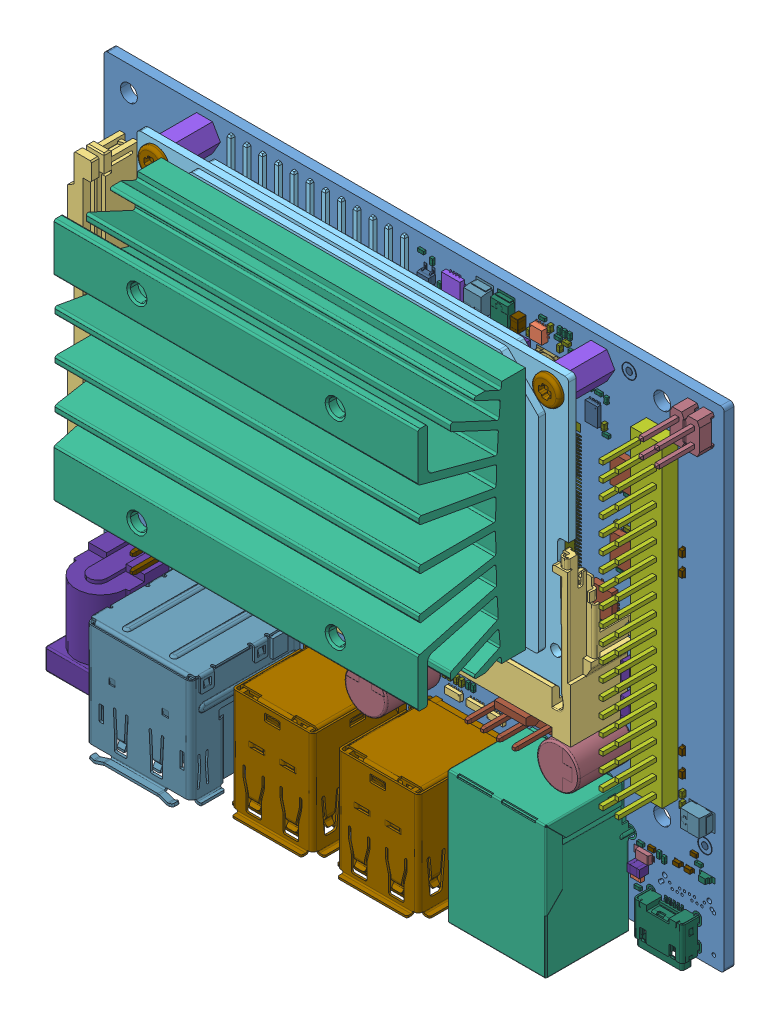
SolidWorks assembly Jetson_Nano_Dev_Kit_3D_b01, configuration Default. Lengths in mm. (continued)
Components (placement in the parent): (continued)
- Jetson_Nano_Dev_Kit_3D_b01(2)^Jetson_Nano_Dev_Kit_3D_b01-1: Jetson_Nano_Dev_Kit_3D_b01(2)^Jetson_Nano_Dev_Kit_3D_b01 [Default] at origin size (100 81.03 30.51) (virtual) (continued)
  - 642-13450_PORG_SYS_BOM^Jetson_Nano_Dev_Kit_3D_b01(2)_Jetson_Nano_Dev_Kit_3D_b01-1: 642-13450_PORG_SYS_BOM^Jetson_Nano_Dev_Kit_3D_b01(2)_Jetson_Nano_Dev_Kit_3D_b01 [Default] at origin size (100 81.03 23.18) (virtual) (continued)
    - 699-13449_PORG_DEV_KIT_PCB_ASSY^642-13450_PORG_SYS_BOM_Jetson_Nano_Dev_Kit_3D_b01(2)_Jetson_Nano_Dev_Kit_3D_b01-1: 699-13449_PORG_DEV_KIT_PCB_ASSY^642-13450_PORG_SYS_BOM_Jetson_Nano_Dev_Kit_3D_b01(2)_Jetson_Nano_Dev_Kit_3D_b01 [Default] at origin size (100 81.03 23.18) (virtual) (continued)
      - 600-13449_PORG_DEV_KIT_PCB_ASSY^699-13449_PORG_DEV_KIT_PCB_ASSY_642-13450_PORG_SYS_BOM_Jetson_Nano_Dev_Kit_3D_b01(2)_Jetson_Nano_Dev_Kit_3D_b01-1: 600-13449_PORG_DEV_KIT_PCB_ASSY^699-13449_PORG_DEV_KIT_PCB_ASSY_642-13450_PORG_SYS_BOM_Jetson_Nano_Dev_Kit_3D_b01(2)_Jetson_Nano_Dev_Kit_3D_b01 [Default] at origin size (100 81.03 23.18) (virtual) (continued)
        - 142-13449-1000-B01-SKU0000^600-13449_PORG_DEV_KIT_PCB_ASSY_699-13449_PORG_DEV_KIT_PCB_ASSY_642-13450_PORG_SYS_BOM_Jetson_Nano_Dev_Kit_3D_b01(2)_Jetson_Nano_Dev_Kit_3D_b01-1: 142-13449-1000-B01-SKU0000^600-13449_PORG_DEV_KIT_PCB_ASSY_699-13449_PORG_DEV_KIT_PCB_ASSY_642-13450_PORG_SYS_BOM_Jetson_Nano_Dev_Kit_3D_b01(2)_Jetson_Nano_Dev_Kit_3D_b01 [Default] at origin size (100 81.03 23.18) (virtual) (continued)
          - 0402_H060^142-13449-1000-B01-SKU0000_600-13449_PORG_DEV_KIT_PCB_ASSY_699-13449_PORG_DEV_KIT_PCB_ASSY_642-13450_PORG_SYS_BOM_Jetson_Nano_Dev_Kit_3D_b01(2)_Jetson_Nano_Dev_Kit_3D_b01-14: 0402_H060^142-13449-1000-B01-SKU0000_600-13449_PORG_DEV_KIT_PCB_ASSY_699-13449_PORG_DEV_KIT_PCB_ASSY_642-13450_PORG_SYS_BOM_Jetson_Nano_Dev_Kit_3D_b01(2)_Jetson_Nano_Dev_Kit_3D_b01 [Default] at (18.6 7.7 1.57) x (0 -1 0) z (0 0 1) size (1 0.5 0.6) (virtual)
          - 0402_H060^142-13449-1000-B01-SKU0000_600-13449_PORG_DEV_KIT_PCB_ASSY_699-13449_PORG_DEV_KIT_PCB_ASSY_642-13450_PORG_SYS_BOM_Jetson_Nano_Dev_Kit_3D_b01(2)_Jetson_Nano_Dev_Kit_3D_b01-15: 0402_H060^142-13449-1000-B01-SKU0000_600-13449_PORG_DEV_KIT_PCB_ASSY_699-13449_PORG_DEV_KIT_PCB_ASSY_642-13450_PORG_SYS_BOM_Jetson_Nano_Dev_Kit_3D_b01(2)_Jetson_Nano_Dev_Kit_3D_b01 [Default] at (12.9 7.7 1.57) x (0 -1 0) z (0 0 1) size (1 0.5 0.6) (virtual)
          - 0402_H060^142-13449-1000-B01-SKU0000_600-13449_PORG_DEV_KIT_PCB_ASSY_699-13449_PORG_DEV_KIT_PCB_ASSY_642-13450_PORG_SYS_BOM_Jetson_Nano_Dev_Kit_3D_b01(2)_Jetson_Nano_Dev_Kit_3D_b01-16: 0402_H060^142-13449-1000-B01-SKU0000_600-13449_PORG_DEV_KIT_PCB_ASSY_699-13449_PORG_DEV_KIT_PCB_ASSY_642-13450_PORG_SYS_BOM_Jetson_Nano_Dev_Kit_3D_b01(2)_Jetson_Nano_Dev_Kit_3D_b01 [Default] at (80.9 37.7 1.57) x (-1 0 0) z (0 0 1) size (1 0.5 0.6) (virtual)
          - 0402_H040^142-13449-1000-B01-SKU0000_600-13449_PORG_DEV_KIT_PCB_ASSY_699-13449_PORG_DEV_KIT_PCB_ASSY_642-13450_PORG_SYS_BOM_Jetson_Nano_Dev_Kit_3D_b01(2)_Jetson_Nano_Dev_Kit_3D_b01-45: 0402_H040^142-13449-1000-B01-SKU0000_600-13449_PORG_DEV_KIT_PCB_ASSY_699-13449_PORG_DEV_KIT_PCB_ASSY_642-13450_PORG_SYS_BOM_Jetson_Nano_Dev_Kit_3D_b01(2)_Jetson_Nano_Dev_Kit_3D_b01 [Default] at (79.5 31.3 1.57) size (1 0.5 0.4) (virtual)
          - 0402_H040^142-13449-1000-B01-SKU0000_600-13449_PORG_DEV_KIT_PCB_ASSY_699-13449_PORG_DEV_KIT_PCB_ASSY_642-13450_PORG_SYS_BOM_Jetson_Nano_Dev_Kit_3D_b01(2)_Jetson_Nano_Dev_Kit_3D_b01-46: 0402_H040^142-13449-1000-B01-SKU0000_600-13449_PORG_DEV_KIT_PCB_ASSY_699-13449_PORG_DEV_KIT_PCB_ASSY_642-13450_PORG_SYS_BOM_Jetson_Nano_Dev_Kit_3D_b01(2)_Jetson_Nano_Dev_Kit_3D_b01 [Default] at (81 31.3 1.57) x (-1 0 0) z (0 0 1) size (1 0.5 0.4) (virtual)
          - 0402_H060^142-13449-1000-B01-SKU0000_600-13449_PORG_DEV_KIT_PCB_ASSY_699-13449_PORG_DEV_KIT_PCB_ASSY_642-13450_PORG_SYS_BOM_Jetson_Nano_Dev_Kit_3D_b01(2)_Jetson_Nano_Dev_Kit_3D_b01-17: 0402_H060^142-13449-1000-B01-SKU0000_600-13449_PORG_DEV_KIT_PCB_ASSY_699-13449_PORG_DEV_KIT_PCB_ASSY_642-13450_PORG_SYS_BOM_Jetson_Nano_Dev_Kit_3D_b01(2)_Jetson_Nano_Dev_Kit_3D_b01 [Default] at (79.3 37.7 1.57) size (1 0.5 0.6) (virtual)
          - 0402_H060^142-13449-1000-B01-SKU0000_600-13449_PORG_DEV_KIT_PCB_ASSY_699-13449_PORG_DEV_KIT_PCB_ASSY_642-13450_PORG_SYS_BOM_Jetson_Nano_Dev_Kit_3D_b01(2)_Jetson_Nano_Dev_Kit_3D_b01-18: 0402_H060^142-13449-1000-B01-SKU0000_600-13449_PORG_DEV_KIT_PCB_ASSY_699-13449_PORG_DEV_KIT_PCB_ASSY_642-13450_PORG_SYS_BOM_Jetson_Nano_Dev_Kit_3D_b01(2)_Jetson_Nano_Dev_Kit_3D_b01 [Default] at (74.1 7.6 1.57) x (0 -1 0) z (0 0 1) size (1 0.5 0.6) (virtual)
          - 0402_H040^142-13449-1000-B01-SKU0000_600-13449_PORG_DEV_KIT_PCB_ASSY_699-13449_PORG_DEV_KIT_PCB_ASSY_642-13450_PORG_SYS_BOM_Jetson_Nano_Dev_Kit_3D_b01(2)_Jetson_Nano_Dev_Kit_3D_b01-47: 0402_H040^142-13449-1000-B01-SKU0000_600-13449_PORG_DEV_KIT_PCB_ASSY_699-13449_PORG_DEV_KIT_PCB_ASSY_642-13450_PORG_SYS_BOM_Jetson_Nano_Dev_Kit_3D_b01(2)_Jetson_Nano_Dev_Kit_3D_b01 [Default] at (62.25 4.8 1.57) x (0 -1 0) z (0 0 1) size (1 0.5 0.4) (virtual)
          - 0402_H060^142-13449-1000-B01-SKU0000_600-13449_PORG_DEV_KIT_PCB_ASSY_699-13449_PORG_DEV_KIT_PCB_ASSY_642-13450_PORG_SYS_BOM_Jetson_Nano_Dev_Kit_3D_b01(2)_Jetson_Nano_Dev_Kit_3D_b01-19: 0402_H060^142-13449-1000-B01-SKU0000_600-13449_PORG_DEV_KIT_PCB_ASSY_699-13449_PORG_DEV_KIT_PCB_ASSY_642-13450_PORG_SYS_BOM_Jetson_Nano_Dev_Kit_3D_b01(2)_Jetson_Nano_Dev_Kit_3D_b01 [Default] at (68.35 59.55 1.57) x (0 -1 0) z (0 0 1) size (1 0.5 0.6) (virtual)
          - 0402_H060^142-13449-1000-B01-SKU0000_600-13449_PORG_DEV_KIT_PCB_ASSY_699-13449_PORG_DEV_KIT_PCB_ASSY_642-13450_PORG_SYS_BOM_Jetson_Nano_Dev_Kit_3D_b01(2)_Jetson_Nano_Dev_Kit_3D_b01-20: 0402_H060^142-13449-1000-B01-SKU0000_600-13449_PORG_DEV_KIT_PCB_ASSY_699-13449_PORG_DEV_KIT_PCB_ASSY_642-13450_PORG_SYS_BOM_Jetson_Nano_Dev_Kit_3D_b01(2)_Jetson_Nano_Dev_Kit_3D_b01 [Default] at (17.1 37.95 1.57) x (-1 0 0) z (0 0 1) size (1 0.5 0.6) (virtual)
          - 0402_H060^142-13449-1000-B01-SKU0000_600-13449_PORG_DEV_KIT_PCB_ASSY_699-13449_PORG_DEV_KIT_PCB_ASSY_642-13450_PORG_SYS_BOM_Jetson_Nano_Dev_Kit_3D_b01(2)_Jetson_Nano_Dev_Kit_3D_b01-21: 0402_H060^142-13449-1000-B01-SKU0000_600-13449_PORG_DEV_KIT_PCB_ASSY_699-13449_PORG_DEV_KIT_PCB_ASSY_642-13450_PORG_SYS_BOM_Jetson_Nano_Dev_Kit_3D_b01(2)_Jetson_Nano_Dev_Kit_3D_b01 [Default] at (53.25 2.9 1.57) x (0 -1 0) z (0 0 1) size (1 0.5 0.6) (virtual)
          - 0402_H060^142-13449-1000-B01-SKU0000_600-13449_PORG_DEV_KIT_PCB_ASSY_699-13449_PORG_DEV_KIT_PCB_ASSY_642-13450_PORG_SYS_BOM_Jetson_Nano_Dev_Kit_3D_b01(2)_Jetson_Nano_Dev_Kit_3D_b01-22: 0402_H060^142-13449-1000-B01-SKU0000_600-13449_PORG_DEV_KIT_PCB_ASSY_699-13449_PORG_DEV_KIT_PCB_ASSY_642-13450_PORG_SYS_BOM_Jetson_Nano_Dev_Kit_3D_b01(2)_Jetson_Nano_Dev_Kit_3D_b01 [Default] at (20.85 41.4 1.57) x (-1 0 0) z (0 0 1) size (1 0.5 0.6) (virtual)
          - 0402_H060^142-13449-1000-B01-SKU0000_600-13449_PORG_DEV_KIT_PCB_ASSY_699-13449_PORG_DEV_KIT_PCB_ASSY_642-13450_PORG_SYS_BOM_Jetson_Nano_Dev_Kit_3D_b01(2)_Jetson_Nano_Dev_Kit_3D_b01-23: 0402_H060^142-13449-1000-B01-SKU0000_600-13449_PORG_DEV_KIT_PCB_ASSY_699-13449_PORG_DEV_KIT_PCB_ASSY_642-13450_PORG_SYS_BOM_Jetson_Nano_Dev_Kit_3D_b01(2)_Jetson_Nano_Dev_Kit_3D_b01 [Default] at (19.05 41.4 1.57) x (-1 0 0) z (0 0 1) size (1 0.5 0.6) (virtual)
          - 0402_H060^142-13449-1000-B01-SKU0000_600-13449_PORG_DEV_KIT_PCB_ASSY_699-13449_PORG_DEV_KIT_PCB_ASSY_642-13450_PORG_SYS_BOM_Jetson_Nano_Dev_Kit_3D_b01(2)_Jetson_Nano_Dev_Kit_3D_b01-24: 0402_H060^142-13449-1000-B01-SKU0000_600-13449_PORG_DEV_KIT_PCB_ASSY_699-13449_PORG_DEV_KIT_PCB_ASSY_642-13450_PORG_SYS_BOM_Jetson_Nano_Dev_Kit_3D_b01(2)_Jetson_Nano_Dev_Kit_3D_b01 [Default] at (20.45 28.55 1.57) x (0 -1 0) z (0 0 1) size (1 0.5 0.6) (virtual)
          - 0402_H060^142-13449-1000-B01-SKU0000_600-13449_PORG_DEV_KIT_PCB_ASSY_699-13449_PORG_DEV_KIT_PCB_ASSY_642-13450_PORG_SYS_BOM_Jetson_Nano_Dev_Kit_3D_b01(2)_Jetson_Nano_Dev_Kit_3D_b01-25: 0402_H060^142-13449-1000-B01-SKU0000_600-13449_PORG_DEV_KIT_PCB_ASSY_699-13449_PORG_DEV_KIT_PCB_ASSY_642-13450_PORG_SYS_BOM_Jetson_Nano_Dev_Kit_3D_b01(2)_Jetson_Nano_Dev_Kit_3D_b01 [Default] at (19.55 28.55 1.57) x (0 -1 0) z (0 0 1) size (1 0.5 0.6) (virtual)
          - 0402_H060^142-13449-1000-B01-SKU0000_600-13449_PORG_DEV_KIT_PCB_ASSY_699-13449_PORG_DEV_KIT_PCB_ASSY_642-13450_PORG_SYS_BOM_Jetson_Nano_Dev_Kit_3D_b01(2)_Jetson_Nano_Dev_Kit_3D_b01-26: 0402_H060^142-13449-1000-B01-SKU0000_600-13449_PORG_DEV_KIT_PCB_ASSY_699-13449_PORG_DEV_KIT_PCB_ASSY_642-13450_PORG_SYS_BOM_Jetson_Nano_Dev_Kit_3D_b01(2)_Jetson_Nano_Dev_Kit_3D_b01 [Default] at (54.05 2.9 1.57) x (0 -1 0) z (0 0 1) size (1 0.5 0.6) (virtual)
          - 0402_H060^142-13449-1000-B01-SKU0000_600-13449_PORG_DEV_KIT_PCB_ASSY_699-13449_PORG_DEV_KIT_PCB_ASSY_642-13450_PORG_SYS_BOM_Jetson_Nano_Dev_Kit_3D_b01(2)_Jetson_Nano_Dev_Kit_3D_b01-27: 0402_H060^142-13449-1000-B01-SKU0000_600-13449_PORG_DEV_KIT_PCB_ASSY_699-13449_PORG_DEV_KIT_PCB_ASSY_642-13450_PORG_SYS_BOM_Jetson_Nano_Dev_Kit_3D_b01(2)_Jetson_Nano_Dev_Kit_3D_b01 [Default] at (22.5 28.58 1.57) x (0 -1 0) z (0 0 1) size (1 0.5 0.6) (virtual)
          - 0402_H040^142-13449-1000-B01-SKU0000_600-13449_PORG_DEV_KIT_PCB_ASSY_699-13449_PORG_DEV_KIT_PCB_ASSY_642-13450_PORG_SYS_BOM_Jetson_Nano_Dev_Kit_3D_b01(2)_Jetson_Nano_Dev_Kit_3D_b01-48: 0402_H040^142-13449-1000-B01-SKU0000_600-13449_PORG_DEV_KIT_PCB_ASSY_699-13449_PORG_DEV_KIT_PCB_ASSY_642-13450_PORG_SYS_BOM_Jetson_Nano_Dev_Kit_3D_b01(2)_Jetson_Nano_Dev_Kit_3D_b01 [Default] at (55.8 2.95 1.57) x (0 -1 0) z (0 0 1) size (1 0.5 0.4) (virtual)
          - 0402_H040^142-13449-1000-B01-SKU0000_600-13449_PORG_DEV_KIT_PCB_ASSY_699-13449_PORG_DEV_KIT_PCB_ASSY_642-13450_PORG_SYS_BOM_Jetson_Nano_Dev_Kit_3D_b01(2)_Jetson_Nano_Dev_Kit_3D_b01-49: 0402_H040^142-13449-1000-B01-SKU0000_600-13449_PORG_DEV_KIT_PCB_ASSY_699-13449_PORG_DEV_KIT_PCB_ASSY_642-13450_PORG_SYS_BOM_Jetson_Nano_Dev_Kit_3D_b01(2)_Jetson_Nano_Dev_Kit_3D_b01 [Default] at (18.63 28.53 1.57) x (0 1 0) z (0 0 1) size (1 0.5 0.4) (virtual)
          - 0402_H060^142-13449-1000-B01-SKU0000_600-13449_PORG_DEV_KIT_PCB_ASSY_699-13449_PORG_DEV_KIT_PCB_ASSY_642-13450_PORG_SYS_BOM_Jetson_Nano_Dev_Kit_3D_b01(2)_Jetson_Nano_Dev_Kit_3D_b01-28: 0402_H060^142-13449-1000-B01-SKU0000_600-13449_PORG_DEV_KIT_PCB_ASSY_699-13449_PORG_DEV_KIT_PCB_ASSY_642-13450_PORG_SYS_BOM_Jetson_Nano_Dev_Kit_3D_b01(2)_Jetson_Nano_Dev_Kit_3D_b01 [Default] at (16.9 29.15 1.57) x (0 1 0) z (0 0 1) size (1 0.5 0.6) (virtual)
          - 0402_H060^142-13449-1000-B01-SKU0000_600-13449_PORG_DEV_KIT_PCB_ASSY_699-13449_PORG_DEV_KIT_PCB_ASSY_642-13450_PORG_SYS_BOM_Jetson_Nano_Dev_Kit_3D_b01(2)_Jetson_Nano_Dev_Kit_3D_b01-29: 0402_H060^142-13449-1000-B01-SKU0000_600-13449_PORG_DEV_KIT_PCB_ASSY_699-13449_PORG_DEV_KIT_PCB_ASSY_642-13450_PORG_SYS_BOM_Jetson_Nano_Dev_Kit_3D_b01(2)_Jetson_Nano_Dev_Kit_3D_b01 [Default] at (16.9 30.75 1.57) x (0 1 0) z (0 0 1) size (1 0.5 0.6) (virtual)
          - 0402_H040^142-13449-1000-B01-SKU0000_600-13449_PORG_DEV_KIT_PCB_ASSY_699-13449_PORG_DEV_KIT_PCB_ASSY_642-13450_PORG_SYS_BOM_Jetson_Nano_Dev_Kit_3D_b01(2)_Jetson_Nano_Dev_Kit_3D_b01-50: 0402_H040^142-13449-1000-B01-SKU0000_600-13449_PORG_DEV_KIT_PCB_ASSY_699-13449_PORG_DEV_KIT_PCB_ASSY_642-13450_PORG_SYS_BOM_Jetson_Nano_Dev_Kit_3D_b01(2)_Jetson_Nano_Dev_Kit_3D_b01 [Default] at (39.6 2.87 1.57) x (0 -1 0) z (0 0 1) size (1 0.5 0.4) (virtual)
          - 0402_H040^142-13449-1000-B01-SKU0000_600-13449_PORG_DEV_KIT_PCB_ASSY_699-13449_PORG_DEV_KIT_PCB_ASSY_642-13450_PORG_SYS_BOM_Jetson_Nano_Dev_Kit_3D_b01(2)_Jetson_Nano_Dev_Kit_3D_b01-51: 0402_H040^142-13449-1000-B01-SKU0000_600-13449_PORG_DEV_KIT_PCB_ASSY_699-13449_PORG_DEV_KIT_PCB_ASSY_642-13450_PORG_SYS_BOM_Jetson_Nano_Dev_Kit_3D_b01(2)_Jetson_Nano_Dev_Kit_3D_b01 [Default] at (40.4 2.87 1.57) x (0 -1 0) z (0 0 1) size (1 0.5 0.4) (virtual)
          - 0402_H040^142-13449-1000-B01-SKU0000_600-13449_PORG_DEV_KIT_PCB_ASSY_699-13449_PORG_DEV_KIT_PCB_ASSY_642-13450_PORG_SYS_BOM_Jetson_Nano_Dev_Kit_3D_b01(2)_Jetson_Nano_Dev_Kit_3D_b01-52: 0402_H040^142-13449-1000-B01-SKU0000_600-13449_PORG_DEV_KIT_PCB_ASSY_699-13449_PORG_DEV_KIT_PCB_ASSY_642-13450_PORG_SYS_BOM_Jetson_Nano_Dev_Kit_3D_b01(2)_Jetson_Nano_Dev_Kit_3D_b01 [Default] at (60.95 2.95 1.57) x (0 -1 0) z (0 0 1) size (1 0.5 0.4) (virtual)
          - 0402_H040^142-13449-1000-B01-SKU0000_600-13449_PORG_DEV_KIT_PCB_ASSY_699-13449_PORG_DEV_KIT_PCB_ASSY_642-13450_PORG_SYS_BOM_Jetson_Nano_Dev_Kit_3D_b01(2)_Jetson_Nano_Dev_Kit_3D_b01-53: 0402_H040^142-13449-1000-B01-SKU0000_600-13449_PORG_DEV_KIT_PCB_ASSY_699-13449_PORG_DEV_KIT_PCB_ASSY_642-13450_PORG_SYS_BOM_Jetson_Nano_Dev_Kit_3D_b01(2)_Jetson_Nano_Dev_Kit_3D_b01 [Default] at (60.15 2.95 1.57) x (0 -1 0) z (0 0 1) size (1 0.5 0.4) (virtual)
          - 0402_H040^142-13449-1000-B01-SKU0000_600-13449_PORG_DEV_KIT_PCB_ASSY_699-13449_PORG_DEV_KIT_PCB_ASSY_642-13450_PORG_SYS_BOM_Jetson_Nano_Dev_Kit_3D_b01(2)_Jetson_Nano_Dev_Kit_3D_b01-54: 0402_H040^142-13449-1000-B01-SKU0000_600-13449_PORG_DEV_KIT_PCB_ASSY_699-13449_PORG_DEV_KIT_PCB_ASSY_642-13450_PORG_SYS_BOM_Jetson_Nano_Dev_Kit_3D_b01(2)_Jetson_Nano_Dev_Kit_3D_b01 [Default] at (55 2.95 1.57) x (0 -1 0) z (0 0 1) size (1 0.5 0.4) (virtual)
          - 0402_H040^142-13449-1000-B01-SKU0000_600-13449_PORG_DEV_KIT_PCB_ASSY_699-13449_PORG_DEV_KIT_PCB_ASSY_642-13450_PORG_SYS_BOM_Jetson_Nano_Dev_Kit_3D_b01(2)_Jetson_Nano_Dev_Kit_3D_b01-55: 0402_H040^142-13449-1000-B01-SKU0000_600-13449_PORG_DEV_KIT_PCB_ASSY_699-13449_PORG_DEV_KIT_PCB_ASSY_642-13450_PORG_SYS_BOM_Jetson_Nano_Dev_Kit_3D_b01(2)_Jetson_Nano_Dev_Kit_3D_b01 [Default] at (63.775 -14.475 1.57) size (1 0.5 0.4) (virtual)
          - 0402_H040^142-13449-1000-B01-SKU0000_600-13449_PORG_DEV_KIT_PCB_ASSY_699-13449_PORG_DEV_KIT_PCB_ASSY_642-13450_PORG_SYS_BOM_Jetson_Nano_Dev_Kit_3D_b01(2)_Jetson_Nano_Dev_Kit_3D_b01-56: 0402_H040^142-13449-1000-B01-SKU0000_600-13449_PORG_DEV_KIT_PCB_ASSY_699-13449_PORG_DEV_KIT_PCB_ASSY_642-13450_PORG_SYS_BOM_Jetson_Nano_Dev_Kit_3D_b01(2)_Jetson_Nano_Dev_Kit_3D_b01 [Default] at (63.775 -15.275 1.57) size (1 0.5 0.4) (virtual)
          - 0402_H040^142-13449-1000-B01-SKU0000_600-13449_PORG_DEV_KIT_PCB_ASSY_699-13449_PORG_DEV_KIT_PCB_ASSY_642-13450_PORG_SYS_BOM_Jetson_Nano_Dev_Kit_3D_b01(2)_Jetson_Nano_Dev_Kit_3D_b01-57: 0402_H040^142-13449-1000-B01-SKU0000_600-13449_PORG_DEV_KIT_PCB_ASSY_699-13449_PORG_DEV_KIT_PCB_ASSY_642-13450_PORG_SYS_BOM_Jetson_Nano_Dev_Kit_3D_b01(2)_Jetson_Nano_Dev_Kit_3D_b01 [Default] at (32.65 42.9 1.57) x (0 1 0) z (0 0 1) size (1 0.5 0.4) (virtual)
          - 0402_H060^142-13449-1000-B01-SKU0000_600-13449_PORG_DEV_KIT_PCB_ASSY_699-13449_PORG_DEV_KIT_PCB_ASSY_642-13450_PORG_SYS_BOM_Jetson_Nano_Dev_Kit_3D_b01(2)_Jetson_Nano_Dev_Kit_3D_b01-30: 0402_H060^142-13449-1000-B01-SKU0000_600-13449_PORG_DEV_KIT_PCB_ASSY_699-13449_PORG_DEV_KIT_PCB_ASSY_642-13450_PORG_SYS_BOM_Jetson_Nano_Dev_Kit_3D_b01(2)_Jetson_Nano_Dev_Kit_3D_b01 [Default] at (63.95 1.25 1.57) x (0 1 0) z (0 0 1) size (1 0.5 0.6) (virtual)
          - 0402_H060^142-13449-1000-B01-SKU0000_600-13449_PORG_DEV_KIT_PCB_ASSY_699-13449_PORG_DEV_KIT_PCB_ASSY_642-13450_PORG_SYS_BOM_Jetson_Nano_Dev_Kit_3D_b01(2)_Jetson_Nano_Dev_Kit_3D_b01-31: 0402_H060^142-13449-1000-B01-SKU0000_600-13449_PORG_DEV_KIT_PCB_ASSY_699-13449_PORG_DEV_KIT_PCB_ASSY_642-13450_PORG_SYS_BOM_Jetson_Nano_Dev_Kit_3D_b01(2)_Jetson_Nano_Dev_Kit_3D_b01 [Default] at (37.8 49.2 1.57) x (0 1 0) z (0 0 1) size (1 0.5 0.6) (virtual)
          - 0402_H040^142-13449-1000-B01-SKU0000_600-13449_PORG_DEV_KIT_PCB_ASSY_699-13449_PORG_DEV_KIT_PCB_ASSY_642-13450_PORG_SYS_BOM_Jetson_Nano_Dev_Kit_3D_b01(2)_Jetson_Nano_Dev_Kit_3D_b01-58: 0402_H040^142-13449-1000-B01-SKU0000_600-13449_PORG_DEV_KIT_PCB_ASSY_699-13449_PORG_DEV_KIT_PCB_ASSY_642-13450_PORG_SYS_BOM_Jetson_Nano_Dev_Kit_3D_b01(2)_Jetson_Nano_Dev_Kit_3D_b01 [Default] at (92.2 -3.45 1.57) x (-1 0 0) z (0 0 1) size (1 0.5 0.4) (virtual)
          - 0402_H060^142-13449-1000-B01-SKU0000_600-13449_PORG_DEV_KIT_PCB_ASSY_699-13449_PORG_DEV_KIT_PCB_ASSY_642-13450_PORG_SYS_BOM_Jetson_Nano_Dev_Kit_3D_b01(2)_Jetson_Nano_Dev_Kit_3D_b01-32: 0402_H060^142-13449-1000-B01-SKU0000_600-13449_PORG_DEV_KIT_PCB_ASSY_699-13449_PORG_DEV_KIT_PCB_ASSY_642-13450_PORG_SYS_BOM_Jetson_Nano_Dev_Kit_3D_b01(2)_Jetson_Nano_Dev_Kit_3D_b01 [Default] at (32.85 7.7 1.57) x (0 -1 0) z (0 0 1) size (1 0.5 0.6) (virtual)
          - 0402_H060^142-13449-1000-B01-SKU0000_600-13449_PORG_DEV_KIT_PCB_ASSY_699-13449_PORG_DEV_KIT_PCB_ASSY_642-13450_PORG_SYS_BOM_Jetson_Nano_Dev_Kit_3D_b01(2)_Jetson_Nano_Dev_Kit_3D_b01-33: 0402_H060^142-13449-1000-B01-SKU0000_600-13449_PORG_DEV_KIT_PCB_ASSY_699-13449_PORG_DEV_KIT_PCB_ASSY_642-13450_PORG_SYS_BOM_Jetson_Nano_Dev_Kit_3D_b01(2)_Jetson_Nano_Dev_Kit_3D_b01 [Default] at (27.25 7.7 1.57) x (0 -1 0) z (0 0 1) size (1 0.5 0.6) (virtual)
          - 0402_H060^142-13449-1000-B01-SKU0000_600-13449_PORG_DEV_KIT_PCB_ASSY_699-13449_PORG_DEV_KIT_PCB_ASSY_642-13450_PORG_SYS_BOM_Jetson_Nano_Dev_Kit_3D_b01(2)_Jetson_Nano_Dev_Kit_3D_b01-34: 0402_H060^142-13449-1000-B01-SKU0000_600-13449_PORG_DEV_KIT_PCB_ASSY_699-13449_PORG_DEV_KIT_PCB_ASSY_642-13450_PORG_SYS_BOM_Jetson_Nano_Dev_Kit_3D_b01(2)_Jetson_Nano_Dev_Kit_3D_b01 [Default] at (31.25 7.7 1.57) x (0 -1 0) z (0 0 1) size (1 0.5 0.6) (virtual)
          - 0402_H060^142-13449-1000-B01-SKU0000_600-13449_PORG_DEV_KIT_PCB_ASSY_699-13449_PORG_DEV_KIT_PCB_ASSY_642-13450_PORG_SYS_BOM_Jetson_Nano_Dev_Kit_3D_b01(2)_Jetson_Nano_Dev_Kit_3D_b01-35: 0402_H060^142-13449-1000-B01-SKU0000_600-13449_PORG_DEV_KIT_PCB_ASSY_699-13449_PORG_DEV_KIT_PCB_ASSY_642-13450_PORG_SYS_BOM_Jetson_Nano_Dev_Kit_3D_b01(2)_Jetson_Nano_Dev_Kit_3D_b01 [Default] at (28.85 7.7 1.57) x (0 -1 0) z (0 0 1) size (1 0.5 0.6) (virtual)
          - 0402_H060^142-13449-1000-B01-SKU0000_600-13449_PORG_DEV_KIT_PCB_ASSY_699-13449_PORG_DEV_KIT_PCB_ASSY_642-13450_PORG_SYS_BOM_Jetson_Nano_Dev_Kit_3D_b01(2)_Jetson_Nano_Dev_Kit_3D_b01-36: 0402_H060^142-13449-1000-B01-SKU0000_600-13449_PORG_DEV_KIT_PCB_ASSY_699-13449_PORG_DEV_KIT_PCB_ASSY_642-13450_PORG_SYS_BOM_Jetson_Nano_Dev_Kit_3D_b01(2)_Jetson_Nano_Dev_Kit_3D_b01 [Default] at (32.05 7.7 1.57) x (0 -1 0) z (0 0 1) size (1 0.5 0.6) (virtual)
          - 0402_H060^142-13449-1000-B01-SKU0000_600-13449_PORG_DEV_KIT_PCB_ASSY_699-13449_PORG_DEV_KIT_PCB_ASSY_642-13450_PORG_SYS_BOM_Jetson_Nano_Dev_Kit_3D_b01(2)_Jetson_Nano_Dev_Kit_3D_b01-37: 0402_H060^142-13449-1000-B01-SKU0000_600-13449_PORG_DEV_KIT_PCB_ASSY_699-13449_PORG_DEV_KIT_PCB_ASSY_642-13450_PORG_SYS_BOM_Jetson_Nano_Dev_Kit_3D_b01(2)_Jetson_Nano_Dev_Kit_3D_b01 [Default] at (28.05 7.7 1.57) x (0 -1 0) z (0 0 1) size (1 0.5 0.6) (virtual)
          - 0402_H060^142-13449-1000-B01-SKU0000_600-13449_PORG_DEV_KIT_PCB_ASSY_699-13449_PORG_DEV_KIT_PCB_ASSY_642-13450_PORG_SYS_BOM_Jetson_Nano_Dev_Kit_3D_b01(2)_Jetson_Nano_Dev_Kit_3D_b01-38: 0402_H060^142-13449-1000-B01-SKU0000_600-13449_PORG_DEV_KIT_PCB_ASSY_699-13449_PORG_DEV_KIT_PCB_ASSY_642-13450_PORG_SYS_BOM_Jetson_Nano_Dev_Kit_3D_b01(2)_Jetson_Nano_Dev_Kit_3D_b01 [Default] at (30.45 7.7 1.57) x (0 -1 0) z (0 0 1) size (1 0.5 0.6) (virtual)
          - 0402_H060^142-13449-1000-B01-SKU0000_600-13449_PORG_DEV_KIT_PCB_ASSY_699-13449_PORG_DEV_KIT_PCB_ASSY_642-13450_PORG_SYS_BOM_Jetson_Nano_Dev_Kit_3D_b01(2)_Jetson_Nano_Dev_Kit_3D_b01-39: 0402_H060^142-13449-1000-B01-SKU0000_600-13449_PORG_DEV_KIT_PCB_ASSY_699-13449_PORG_DEV_KIT_PCB_ASSY_642-13450_PORG_SYS_BOM_Jetson_Nano_Dev_Kit_3D_b01(2)_Jetson_Nano_Dev_Kit_3D_b01 [Default] at (29.65 7.7 1.57) x (0 -1 0) z (0 0 1) size (1 0.5 0.6) (virtual)
          - 0402_H060^142-13449-1000-B01-SKU0000_600-13449_PORG_DEV_KIT_PCB_ASSY_699-13449_PORG_DEV_KIT_PCB_ASSY_642-13450_PORG_SYS_BOM_Jetson_Nano_Dev_Kit_3D_b01(2)_Jetson_Nano_Dev_Kit_3D_b01-40: 0402_H060^142-13449-1000-B01-SKU0000_600-13449_PORG_DEV_KIT_PCB_ASSY_699-13449_PORG_DEV_KIT_PCB_ASSY_642-13450_PORG_SYS_BOM_Jetson_Nano_Dev_Kit_3D_b01(2)_Jetson_Nano_Dev_Kit_3D_b01 [Default] at (24.65 6.41 1.57) x (0 -1 0) z (0 0 1) size (1 0.5 0.6) (virtual)
          - 0402_H060^142-13449-1000-B01-SKU0000_600-13449_PORG_DEV_KIT_PCB_ASSY_699-13449_PORG_DEV_KIT_PCB_ASSY_642-13450_PORG_SYS_BOM_Jetson_Nano_Dev_Kit_3D_b01(2)_Jetson_Nano_Dev_Kit_3D_b01-41: 0402_H060^142-13449-1000-B01-SKU0000_600-13449_PORG_DEV_KIT_PCB_ASSY_699-13449_PORG_DEV_KIT_PCB_ASSY_642-13450_PORG_SYS_BOM_Jetson_Nano_Dev_Kit_3D_b01(2)_Jetson_Nano_Dev_Kit_3D_b01 [Default] at (25.85 6.41 1.57) x (0 -1 0) z (0 0 1) size (1 0.5 0.6) (virtual)
          - 0402_H060^142-13449-1000-B01-SKU0000_600-13449_PORG_DEV_KIT_PCB_ASSY_699-13449_PORG_DEV_KIT_PCB_ASSY_642-13450_PORG_SYS_BOM_Jetson_Nano_Dev_Kit_3D_b01(2)_Jetson_Nano_Dev_Kit_3D_b01-42: 0402_H060^142-13449-1000-B01-SKU0000_600-13449_PORG_DEV_KIT_PCB_ASSY_699-13449_PORG_DEV_KIT_PCB_ASSY_642-13450_PORG_SYS_BOM_Jetson_Nano_Dev_Kit_3D_b01(2)_Jetson_Nano_Dev_Kit_3D_b01 [Default] at (3.8 25.4 1.57) x (0 1 0) z (0 0 1) size (1 0.5 0.6) (virtual)
          - 0402_H060^142-13449-1000-B01-SKU0000_600-13449_PORG_DEV_KIT_PCB_ASSY_699-13449_PORG_DEV_KIT_PCB_ASSY_642-13450_PORG_SYS_BOM_Jetson_Nano_Dev_Kit_3D_b01(2)_Jetson_Nano_Dev_Kit_3D_b01-43: 0402_H060^142-13449-1000-B01-SKU0000_600-13449_PORG_DEV_KIT_PCB_ASSY_699-13449_PORG_DEV_KIT_PCB_ASSY_642-13450_PORG_SYS_BOM_Jetson_Nano_Dev_Kit_3D_b01(2)_Jetson_Nano_Dev_Kit_3D_b01 [Default] at (89.65 5.15 1.57) x (0 -1 0) z (0 0 1) size (1 0.5 0.6) (virtual)
          - 0402_H060^142-13449-1000-B01-SKU0000_600-13449_PORG_DEV_KIT_PCB_ASSY_699-13449_PORG_DEV_KIT_PCB_ASSY_642-13450_PORG_SYS_BOM_Jetson_Nano_Dev_Kit_3D_b01(2)_Jetson_Nano_Dev_Kit_3D_b01-44: 0402_H060^142-13449-1000-B01-SKU0000_600-13449_PORG_DEV_KIT_PCB_ASSY_699-13449_PORG_DEV_KIT_PCB_ASSY_642-13450_PORG_SYS_BOM_Jetson_Nano_Dev_Kit_3D_b01(2)_Jetson_Nano_Dev_Kit_3D_b01 [Default] at (89.65 3.65 1.57) x (0 1 0) z (0 0 1) size (1 0.5 0.6) (virtual)
          - 0402_H060^142-13449-1000-B01-SKU0000_600-13449_PORG_DEV_KIT_PCB_ASSY_699-13449_PORG_DEV_KIT_PCB_ASSY_642-13450_PORG_SYS_BOM_Jetson_Nano_Dev_Kit_3D_b01(2)_Jetson_Nano_Dev_Kit_3D_b01-45: 0402_H060^142-13449-1000-B01-SKU0000_600-13449_PORG_DEV_KIT_PCB_ASSY_699-13449_PORG_DEV_KIT_PCB_ASSY_642-13450_PORG_SYS_BOM_Jetson_Nano_Dev_Kit_3D_b01(2)_Jetson_Nano_Dev_Kit_3D_b01 [Default] at (40.6 44.45 1.57) x (0 1 0) z (0 0 1) size (1 0.5 0.6) (virtual)
          - 0402_H060^142-13449-1000-B01-SKU0000_600-13449_PORG_DEV_KIT_PCB_ASSY_699-13449_PORG_DEV_KIT_PCB_ASSY_642-13450_PORG_SYS_BOM_Jetson_Nano_Dev_Kit_3D_b01(2)_Jetson_Nano_Dev_Kit_3D_b01-46: 0402_H060^142-13449-1000-B01-SKU0000_600-13449_PORG_DEV_KIT_PCB_ASSY_699-13449_PORG_DEV_KIT_PCB_ASSY_642-13450_PORG_SYS_BOM_Jetson_Nano_Dev_Kit_3D_b01(2)_Jetson_Nano_Dev_Kit_3D_b01 [Default] at (38.6 49.2 1.57) x (0 1 0) z (0 0 1) size (1 0.5 0.6) (virtual)
          - 0402_H060^142-13449-1000-B01-SKU0000_600-13449_PORG_DEV_KIT_PCB_ASSY_699-13449_PORG_DEV_KIT_PCB_ASSY_642-13450_PORG_SYS_BOM_Jetson_Nano_Dev_Kit_3D_b01(2)_Jetson_Nano_Dev_Kit_3D_b01-47: 0402_H060^142-13449-1000-B01-SKU0000_600-13449_PORG_DEV_KIT_PCB_ASSY_699-13449_PORG_DEV_KIT_PCB_ASSY_642-13450_PORG_SYS_BOM_Jetson_Nano_Dev_Kit_3D_b01(2)_Jetson_Nano_Dev_Kit_3D_b01 [Default] at (25 29.2 1.57) x (0 -1 0) z (0 0 1) size (1 0.5 0.6) (virtual)
          - 0402_H060^142-13449-1000-B01-SKU0000_600-13449_PORG_DEV_KIT_PCB_ASSY_699-13449_PORG_DEV_KIT_PCB_ASSY_642-13450_PORG_SYS_BOM_Jetson_Nano_Dev_Kit_3D_b01(2)_Jetson_Nano_Dev_Kit_3D_b01-48: 0402_H060^142-13449-1000-B01-SKU0000_600-13449_PORG_DEV_KIT_PCB_ASSY_699-13449_PORG_DEV_KIT_PCB_ASSY_642-13450_PORG_SYS_BOM_Jetson_Nano_Dev_Kit_3D_b01(2)_Jetson_Nano_Dev_Kit_3D_b01 [Default] at (28.65 29.6 1.57) size (1 0.5 0.6) (virtual)
          - 0402_H060^142-13449-1000-B01-SKU0000_600-13449_PORG_DEV_KIT_PCB_ASSY_699-13449_PORG_DEV_KIT_PCB_ASSY_642-13450_PORG_SYS_BOM_Jetson_Nano_Dev_Kit_3D_b01(2)_Jetson_Nano_Dev_Kit_3D_b01-49: 0402_H060^142-13449-1000-B01-SKU0000_600-13449_PORG_DEV_KIT_PCB_ASSY_699-13449_PORG_DEV_KIT_PCB_ASSY_642-13450_PORG_SYS_BOM_Jetson_Nano_Dev_Kit_3D_b01(2)_Jetson_Nano_Dev_Kit_3D_b01 [Default] at (30.2 34.15 1.57) x (0 1 0) z (0 0 1) size (1 0.5 0.6) (virtual)
          - 0402_H060^142-13449-1000-B01-SKU0000_600-13449_PORG_DEV_KIT_PCB_ASSY_699-13449_PORG_DEV_KIT_PCB_ASSY_642-13450_PORG_SYS_BOM_Jetson_Nano_Dev_Kit_3D_b01(2)_Jetson_Nano_Dev_Kit_3D_b01-50: 0402_H060^142-13449-1000-B01-SKU0000_600-13449_PORG_DEV_KIT_PCB_ASSY_699-13449_PORG_DEV_KIT_PCB_ASSY_642-13450_PORG_SYS_BOM_Jetson_Nano_Dev_Kit_3D_b01(2)_Jetson_Nano_Dev_Kit_3D_b01 [Default] at (29.65 36.5 1.57) x (0 1 0) z (0 0 1) size (1 0.5 0.6) (virtual)
          - 0402_H060^142-13449-1000-B01-SKU0000_600-13449_PORG_DEV_KIT_PCB_ASSY_699-13449_PORG_DEV_KIT_PCB_ASSY_642-13450_PORG_SYS_BOM_Jetson_Nano_Dev_Kit_3D_b01(2)_Jetson_Nano_Dev_Kit_3D_b01-51: 0402_H060^142-13449-1000-B01-SKU0000_600-13449_PORG_DEV_KIT_PCB_ASSY_699-13449_PORG_DEV_KIT_PCB_ASSY_642-13450_PORG_SYS_BOM_Jetson_Nano_Dev_Kit_3D_b01(2)_Jetson_Nano_Dev_Kit_3D_b01 [Default] at (17.7 41.05 1.57) x (0 1 0) z (0 0 1) size (1 0.5 0.6) (virtual)
          - 0402_H060^142-13449-1000-B01-SKU0000_600-13449_PORG_DEV_KIT_PCB_ASSY_699-13449_PORG_DEV_KIT_PCB_ASSY_642-13450_PORG_SYS_BOM_Jetson_Nano_Dev_Kit_3D_b01(2)_Jetson_Nano_Dev_Kit_3D_b01-52: 0402_H060^142-13449-1000-B01-SKU0000_600-13449_PORG_DEV_KIT_PCB_ASSY_699-13449_PORG_DEV_KIT_PCB_ASSY_642-13450_PORG_SYS_BOM_Jetson_Nano_Dev_Kit_3D_b01(2)_Jetson_Nano_Dev_Kit_3D_b01 [Default] at (16.45 36 1.57) x (0 -1 0) z (0 0 1) size (1 0.5 0.6) (virtual)
          - 0402_H060^142-13449-1000-B01-SKU0000_600-13449_PORG_DEV_KIT_PCB_ASSY_699-13449_PORG_DEV_KIT_PCB_ASSY_642-13450_PORG_SYS_BOM_Jetson_Nano_Dev_Kit_3D_b01(2)_Jetson_Nano_Dev_Kit_3D_b01-53: 0402_H060^142-13449-1000-B01-SKU0000_600-13449_PORG_DEV_KIT_PCB_ASSY_699-13449_PORG_DEV_KIT_PCB_ASSY_642-13450_PORG_SYS_BOM_Jetson_Nano_Dev_Kit_3D_b01(2)_Jetson_Nano_Dev_Kit_3D_b01 [Default] at (26 41.7 1.57) x (0 1 0) z (0 0 1) size (1 0.5 0.6) (virtual)
          - 0402_H060^142-13449-1000-B01-SKU0000_600-13449_PORG_DEV_KIT_PCB_ASSY_699-13449_PORG_DEV_KIT_PCB_ASSY_642-13450_PORG_SYS_BOM_Jetson_Nano_Dev_Kit_3D_b01(2)_Jetson_Nano_Dev_Kit_3D_b01-54: 0402_H060^142-13449-1000-B01-SKU0000_600-13449_PORG_DEV_KIT_PCB_ASSY_699-13449_PORG_DEV_KIT_PCB_ASSY_642-13450_PORG_SYS_BOM_Jetson_Nano_Dev_Kit_3D_b01(2)_Jetson_Nano_Dev_Kit_3D_b01 [Default] at (30.2 31.85 1.57) x (0 -1 0) z (0 0 1) size (1 0.5 0.6) (virtual)
          - 0402_H060^142-13449-1000-B01-SKU0000_600-13449_PORG_DEV_KIT_PCB_ASSY_699-13449_PORG_DEV_KIT_PCB_ASSY_642-13450_PORG_SYS_BOM_Jetson_Nano_Dev_Kit_3D_b01(2)_Jetson_Nano_Dev_Kit_3D_b01-55: 0402_H060^142-13449-1000-B01-SKU0000_600-13449_PORG_DEV_KIT_PCB_ASSY_699-13449_PORG_DEV_KIT_PCB_ASSY_642-13450_PORG_SYS_BOM_Jetson_Nano_Dev_Kit_3D_b01(2)_Jetson_Nano_Dev_Kit_3D_b01 [Default] at (26.8 41.7 1.57) x (0 1 0) z (0 0 1) size (1 0.5 0.6) (virtual)
          - 0402_H060^142-13449-1000-B01-SKU0000_600-13449_PORG_DEV_KIT_PCB_ASSY_699-13449_PORG_DEV_KIT_PCB_ASSY_642-13450_PORG_SYS_BOM_Jetson_Nano_Dev_Kit_3D_b01(2)_Jetson_Nano_Dev_Kit_3D_b01-56: 0402_H060^142-13449-1000-B01-SKU0000_600-13449_PORG_DEV_KIT_PCB_ASSY_699-13449_PORG_DEV_KIT_PCB_ASSY_642-13450_PORG_SYS_BOM_Jetson_Nano_Dev_Kit_3D_b01(2)_Jetson_Nano_Dev_Kit_3D_b01 [Default] at (17.3 32.75 1.57) x (-1 0 0) z (0 0 1) size (1 0.5 0.6) (virtual)
          - 0402_H060^142-13449-1000-B01-SKU0000_600-13449_PORG_DEV_KIT_PCB_ASSY_699-13449_PORG_DEV_KIT_PCB_ASSY_642-13450_PORG_SYS_BOM_Jetson_Nano_Dev_Kit_3D_b01(2)_Jetson_Nano_Dev_Kit_3D_b01-57: 0402_H060^142-13449-1000-B01-SKU0000_600-13449_PORG_DEV_KIT_PCB_ASSY_699-13449_PORG_DEV_KIT_PCB_ASSY_642-13450_PORG_SYS_BOM_Jetson_Nano_Dev_Kit_3D_b01(2)_Jetson_Nano_Dev_Kit_3D_b01 [Default] at (34.1 2.9 1.57) x (0 -1 0) z (0 0 1) size (1 0.5 0.6) (virtual)
          - 0402_H060^142-13449-1000-B01-SKU0000_600-13449_PORG_DEV_KIT_PCB_ASSY_699-13449_PORG_DEV_KIT_PCB_ASSY_642-13450_PORG_SYS_BOM_Jetson_Nano_Dev_Kit_3D_b01(2)_Jetson_Nano_Dev_Kit_3D_b01-58: 0402_H060^142-13449-1000-B01-SKU0000_600-13449_PORG_DEV_KIT_PCB_ASSY_699-13449_PORG_DEV_KIT_PCB_ASSY_642-13450_PORG_SYS_BOM_Jetson_Nano_Dev_Kit_3D_b01(2)_Jetson_Nano_Dev_Kit_3D_b01 [Default] at (35.8 2.9 1.57) x (0 -1 0) z (0 0 1) size (1 0.5 0.6) (virtual)
          - 0402_H060^142-13449-1000-B01-SKU0000_600-13449_PORG_DEV_KIT_PCB_ASSY_699-13449_PORG_DEV_KIT_PCB_ASSY_642-13450_PORG_SYS_BOM_Jetson_Nano_Dev_Kit_3D_b01(2)_Jetson_Nano_Dev_Kit_3D_b01-59: 0402_H060^142-13449-1000-B01-SKU0000_600-13449_PORG_DEV_KIT_PCB_ASSY_699-13449_PORG_DEV_KIT_PCB_ASSY_642-13450_PORG_SYS_BOM_Jetson_Nano_Dev_Kit_3D_b01(2)_Jetson_Nano_Dev_Kit_3D_b01 [Default] at (34.9 2.9 1.57) x (0 -1 0) z (0 0 1) size (1 0.5 0.6) (virtual)
          - 0402_H060^142-13449-1000-B01-SKU0000_600-13449_PORG_DEV_KIT_PCB_ASSY_699-13449_PORG_DEV_KIT_PCB_ASSY_642-13450_PORG_SYS_BOM_Jetson_Nano_Dev_Kit_3D_b01(2)_Jetson_Nano_Dev_Kit_3D_b01-60: 0402_H060^142-13449-1000-B01-SKU0000_600-13449_PORG_DEV_KIT_PCB_ASSY_699-13449_PORG_DEV_KIT_PCB_ASSY_642-13450_PORG_SYS_BOM_Jetson_Nano_Dev_Kit_3D_b01(2)_Jetson_Nano_Dev_Kit_3D_b01 [Default] at (36.6 2.9 1.57) x (0 -1 0) z (0 0 1) size (1 0.5 0.6) (virtual)
          - 0402_H060^142-13449-1000-B01-SKU0000_600-13449_PORG_DEV_KIT_PCB_ASSY_699-13449_PORG_DEV_KIT_PCB_ASSY_642-13450_PORG_SYS_BOM_Jetson_Nano_Dev_Kit_3D_b01(2)_Jetson_Nano_Dev_Kit_3D_b01-61: 0402_H060^142-13449-1000-B01-SKU0000_600-13449_PORG_DEV_KIT_PCB_ASSY_699-13449_PORG_DEV_KIT_PCB_ASSY_642-13450_PORG_SYS_BOM_Jetson_Nano_Dev_Kit_3D_b01(2)_Jetson_Nano_Dev_Kit_3D_b01 [Default] at (51.45 2.9 1.57) x (0 -1 0) z (0 0 1) size (1 0.5 0.6) (virtual)
          - 0402_H060^142-13449-1000-B01-SKU0000_600-13449_PORG_DEV_KIT_PCB_ASSY_699-13449_PORG_DEV_KIT_PCB_ASSY_642-13450_PORG_SYS_BOM_Jetson_Nano_Dev_Kit_3D_b01(2)_Jetson_Nano_Dev_Kit_3D_b01-62: 0402_H060^142-13449-1000-B01-SKU0000_600-13449_PORG_DEV_KIT_PCB_ASSY_699-13449_PORG_DEV_KIT_PCB_ASSY_642-13450_PORG_SYS_BOM_Jetson_Nano_Dev_Kit_3D_b01(2)_Jetson_Nano_Dev_Kit_3D_b01 [Default] at (52.25 2.9 1.57) x (0 -1 0) z (0 0 1) size (1 0.5 0.6) (virtual)
          - 0402_H060^142-13449-1000-B01-SKU0000_600-13449_PORG_DEV_KIT_PCB_ASSY_699-13449_PORG_DEV_KIT_PCB_ASSY_642-13450_PORG_SYS_BOM_Jetson_Nano_Dev_Kit_3D_b01(2)_Jetson_Nano_Dev_Kit_3D_b01-63: 0402_H060^142-13449-1000-B01-SKU0000_600-13449_PORG_DEV_KIT_PCB_ASSY_699-13449_PORG_DEV_KIT_PCB_ASSY_642-13450_PORG_SYS_BOM_Jetson_Nano_Dev_Kit_3D_b01(2)_Jetson_Nano_Dev_Kit_3D_b01 [Default] at (8.9 -8.55 1.57) x (-1 0 0) z (0 0 1) size (1 0.5 0.6) (virtual)
          - 0402_H060^142-13449-1000-B01-SKU0000_600-13449_PORG_DEV_KIT_PCB_ASSY_699-13449_PORG_DEV_KIT_PCB_ASSY_642-13450_PORG_SYS_BOM_Jetson_Nano_Dev_Kit_3D_b01(2)_Jetson_Nano_Dev_Kit_3D_b01-64: 0402_H060^142-13449-1000-B01-SKU0000_600-13449_PORG_DEV_KIT_PCB_ASSY_699-13449_PORG_DEV_KIT_PCB_ASSY_642-13450_PORG_SYS_BOM_Jetson_Nano_Dev_Kit_3D_b01(2)_Jetson_Nano_Dev_Kit_3D_b01 [Default] at (20.7 47.25 1.57) x (0 -1 0) z (0 0 1) size (1 0.5 0.6) (virtual)
          - 0402_H060^142-13449-1000-B01-SKU0000_600-13449_PORG_DEV_KIT_PCB_ASSY_699-13449_PORG_DEV_KIT_PCB_ASSY_642-13450_PORG_SYS_BOM_Jetson_Nano_Dev_Kit_3D_b01(2)_Jetson_Nano_Dev_Kit_3D_b01-65: 0402_H060^142-13449-1000-B01-SKU0000_600-13449_PORG_DEV_KIT_PCB_ASSY_699-13449_PORG_DEV_KIT_PCB_ASSY_642-13450_PORG_SYS_BOM_Jetson_Nano_Dev_Kit_3D_b01(2)_Jetson_Nano_Dev_Kit_3D_b01 [Default] at (77.05 50.15 1.57) x (0 1 0) z (0 0 1) size (1 0.5 0.6) (virtual)
          - 0402_H060^142-13449-1000-B01-SKU0000_600-13449_PORG_DEV_KIT_PCB_ASSY_699-13449_PORG_DEV_KIT_PCB_ASSY_642-13450_PORG_SYS_BOM_Jetson_Nano_Dev_Kit_3D_b01(2)_Jetson_Nano_Dev_Kit_3D_b01-66: 0402_H060^142-13449-1000-B01-SKU0000_600-13449_PORG_DEV_KIT_PCB_ASSY_699-13449_PORG_DEV_KIT_PCB_ASSY_642-13450_PORG_SYS_BOM_Jetson_Nano_Dev_Kit_3D_b01(2)_Jetson_Nano_Dev_Kit_3D_b01 [Default] at (57.4 38.75 1.57) x (0 -1 0) z (0 0 1) size (1 0.5 0.6) (virtual)
          - 0402_H060^142-13449-1000-B01-SKU0000_600-13449_PORG_DEV_KIT_PCB_ASSY_699-13449_PORG_DEV_KIT_PCB_ASSY_642-13450_PORG_SYS_BOM_Jetson_Nano_Dev_Kit_3D_b01(2)_Jetson_Nano_Dev_Kit_3D_b01-67: 0402_H060^142-13449-1000-B01-SKU0000_600-13449_PORG_DEV_KIT_PCB_ASSY_699-13449_PORG_DEV_KIT_PCB_ASSY_642-13450_PORG_SYS_BOM_Jetson_Nano_Dev_Kit_3D_b01(2)_Jetson_Nano_Dev_Kit_3D_b01 [Default] at (58.2 38.75 1.57) x (0 -1 0) z (0 0 1) size (1 0.5 0.6) (virtual)
          - 0402_H060^142-13449-1000-B01-SKU0000_600-13449_PORG_DEV_KIT_PCB_ASSY_699-13449_PORG_DEV_KIT_PCB_ASSY_642-13450_PORG_SYS_BOM_Jetson_Nano_Dev_Kit_3D_b01(2)_Jetson_Nano_Dev_Kit_3D_b01-68: 0402_H060^142-13449-1000-B01-SKU0000_600-13449_PORG_DEV_KIT_PCB_ASSY_699-13449_PORG_DEV_KIT_PCB_ASSY_642-13450_PORG_SYS_BOM_Jetson_Nano_Dev_Kit_3D_b01(2)_Jetson_Nano_Dev_Kit_3D_b01 [Default] at (17.1 38.85 1.57) size (1 0.5 0.6) (virtual)
          - 0402_H060^142-13449-1000-B01-SKU0000_600-13449_PORG_DEV_KIT_PCB_ASSY_699-13449_PORG_DEV_KIT_PCB_ASSY_642-13450_PORG_SYS_BOM_Jetson_Nano_Dev_Kit_3D_b01(2)_Jetson_Nano_Dev_Kit_3D_b01-69: 0402_H060^142-13449-1000-B01-SKU0000_600-13449_PORG_DEV_KIT_PCB_ASSY_699-13449_PORG_DEV_KIT_PCB_ASSY_642-13450_PORG_SYS_BOM_Jetson_Nano_Dev_Kit_3D_b01(2)_Jetson_Nano_Dev_Kit_3D_b01 [Default] at (17.1 39.65 1.57) size (1 0.5 0.6) (virtual)
          - 0402_H060^142-13449-1000-B01-SKU0000_600-13449_PORG_DEV_KIT_PCB_ASSY_699-13449_PORG_DEV_KIT_PCB_ASSY_642-13450_PORG_SYS_BOM_Jetson_Nano_Dev_Kit_3D_b01(2)_Jetson_Nano_Dev_Kit_3D_b01-70: 0402_H060^142-13449-1000-B01-SKU0000_600-13449_PORG_DEV_KIT_PCB_ASSY_699-13449_PORG_DEV_KIT_PCB_ASSY_642-13450_PORG_SYS_BOM_Jetson_Nano_Dev_Kit_3D_b01(2)_Jetson_Nano_Dev_Kit_3D_b01 [Default] at (15.6 45.6 1.57) x (0 1 0) z (0 0 1) size (1 0.5 0.6) (virtual)
          - 0402_H060^142-13449-1000-B01-SKU0000_600-13449_PORG_DEV_KIT_PCB_ASSY_699-13449_PORG_DEV_KIT_PCB_ASSY_642-13450_PORG_SYS_BOM_Jetson_Nano_Dev_Kit_3D_b01(2)_Jetson_Nano_Dev_Kit_3D_b01-71: 0402_H060^142-13449-1000-B01-SKU0000_600-13449_PORG_DEV_KIT_PCB_ASSY_699-13449_PORG_DEV_KIT_PCB_ASSY_642-13450_PORG_SYS_BOM_Jetson_Nano_Dev_Kit_3D_b01(2)_Jetson_Nano_Dev_Kit_3D_b01 [Default] at (15.1 7.7 1.57) x (0 -1 0) z (0 0 1) size (1 0.5 0.6) (virtual)
          - 0402_H060^142-13449-1000-B01-SKU0000_600-13449_PORG_DEV_KIT_PCB_ASSY_699-13449_PORG_DEV_KIT_PCB_ASSY_642-13450_PORG_SYS_BOM_Jetson_Nano_Dev_Kit_3D_b01(2)_Jetson_Nano_Dev_Kit_3D_b01-72: 0402_H060^142-13449-1000-B01-SKU0000_600-13449_PORG_DEV_KIT_PCB_ASSY_699-13449_PORG_DEV_KIT_PCB_ASSY_642-13450_PORG_SYS_BOM_Jetson_Nano_Dev_Kit_3D_b01(2)_Jetson_Nano_Dev_Kit_3D_b01 [Default] at (16.4 7.7 1.57) x (0 -1 0) z (0 0 1) size (1 0.5 0.6) (virtual)
          - 0402_H060^142-13449-1000-B01-SKU0000_600-13449_PORG_DEV_KIT_PCB_ASSY_699-13449_PORG_DEV_KIT_PCB_ASSY_642-13450_PORG_SYS_BOM_Jetson_Nano_Dev_Kit_3D_b01(2)_Jetson_Nano_Dev_Kit_3D_b01-73: 0402_H060^142-13449-1000-B01-SKU0000_600-13449_PORG_DEV_KIT_PCB_ASSY_699-13449_PORG_DEV_KIT_PCB_ASSY_642-13450_PORG_SYS_BOM_Jetson_Nano_Dev_Kit_3D_b01(2)_Jetson_Nano_Dev_Kit_3D_b01 [Default] at (20.8 7.7 1.57) x (0 -1 0) z (0 0 1) size (1 0.5 0.6) (virtual)
          - 0402_H060^142-13449-1000-B01-SKU0000_600-13449_PORG_DEV_KIT_PCB_ASSY_699-13449_PORG_DEV_KIT_PCB_ASSY_642-13450_PORG_SYS_BOM_Jetson_Nano_Dev_Kit_3D_b01(2)_Jetson_Nano_Dev_Kit_3D_b01-74: 0402_H060^142-13449-1000-B01-SKU0000_600-13449_PORG_DEV_KIT_PCB_ASSY_699-13449_PORG_DEV_KIT_PCB_ASSY_642-13450_PORG_SYS_BOM_Jetson_Nano_Dev_Kit_3D_b01(2)_Jetson_Nano_Dev_Kit_3D_b01 [Default] at (19.5 7.7 1.57) x (0 -1 0) z (0 0 1) size (1 0.5 0.6) (virtual)
          - 0402_H060^142-13449-1000-B01-SKU0000_600-13449_PORG_DEV_KIT_PCB_ASSY_699-13449_PORG_DEV_KIT_PCB_ASSY_642-13450_PORG_SYS_BOM_Jetson_Nano_Dev_Kit_3D_b01(2)_Jetson_Nano_Dev_Kit_3D_b01-75: 0402_H060^142-13449-1000-B01-SKU0000_600-13449_PORG_DEV_KIT_PCB_ASSY_699-13449_PORG_DEV_KIT_PCB_ASSY_642-13450_PORG_SYS_BOM_Jetson_Nano_Dev_Kit_3D_b01(2)_Jetson_Nano_Dev_Kit_3D_b01 [Default] at (21.9 2.8 1.57) size (1 0.5 0.6) (virtual)
          - 0402_H060^142-13449-1000-B01-SKU0000_600-13449_PORG_DEV_KIT_PCB_ASSY_699-13449_PORG_DEV_KIT_PCB_ASSY_642-13450_PORG_SYS_BOM_Jetson_Nano_Dev_Kit_3D_b01(2)_Jetson_Nano_Dev_Kit_3D_b01-76: 0402_H060^142-13449-1000-B01-SKU0000_600-13449_PORG_DEV_KIT_PCB_ASSY_699-13449_PORG_DEV_KIT_PCB_ASSY_642-13450_PORG_SYS_BOM_Jetson_Nano_Dev_Kit_3D_b01(2)_Jetson_Nano_Dev_Kit_3D_b01 [Default] at (9.85 -7.25 1.57) x (-1 0 0) z (0 0 1) size (1 0.5 0.6) (virtual)
